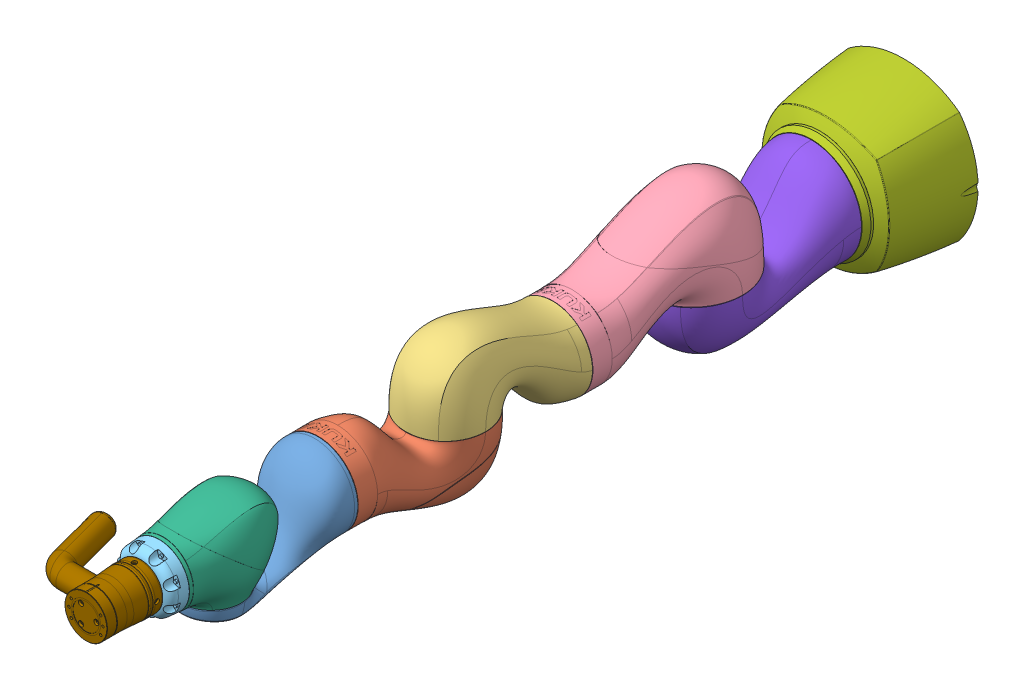
SolidWorks assembly lbrMed_withBaseLink_Frames, configuration Default. Lengths in mm.
Overall size (319.95 277.84 1446.36).
10 component instances, 10 part files, 6 mates.
Components (placement in the parent):
- Wrist1_body-2: Wrist1_body [Default] at origin size (137.43 170.81 261.47)
- UpperArm_body-1: UpperArm_body [Default] at origin size (137.03 183.96 286.04)
- Elbow_body-1: Elbow_body [Default] at origin size (136.09 183.95 261.22)
- LowerArm_body-1: LowerArm_body [Default] at origin size (171.08 201.65 323.93)
- Wrist3_body-1: Wrist3_body [Default] at origin size (102.25 102.25 38.4)
- Wrist2_body-1: Wrist2_body [Default] at origin size (136.25 137.94 182.79)
- Base_body-1: Base_body [Default] at origin size (277.84 277.84 157.78)
- Shoulder_body-1: Shoulder_body [Default] at origin size (171.08 202.96 299.34)
- only_platform-1: only_platform [Default] at (515.1468 0 -732.7058) x (-0.819152 0 -0.573576) z (0 1 0) size (1151.95 1181.08 766) (hidden)
- only_link-1: only_link [Default] at (515.1468 0 -732.7058) x (-0.819152 0 -0.573576) z (0 1 0) size (227.18 131.55 78.48)
Mates (geometry in assembly coordinates):
- Concentric1: concentric aligned: cylinder of Base_body-1 through (84.8528 84.8528 0) axis (0 0 1) radius 5; cylinder of only_platform-1 through (84.8528 84.8528 -125.779) axis (0 0 1) radius 5.25
- Concentric2: concentric aligned: cylinder of Base_body-1 through (84.8528 -84.8528 0) axis (0 0 1) radius 5; cylinder of only_platform-1 through (84.8528 -84.8528 -125.779) axis (0 0 1) radius 5.25
- Coincident1: coincident anti-aligned: plane of Base_body-1 through (0 0 3) normal (0 0 -1); plane of only_platform-1 through (127.5 127.5 3) normal (0 0 1)
- Concentric3: concentric anti-aligned: cylinder of Wrist3_body-1 through (-9.7581 9.7581 1289.3) axis (0 0 1) radius 3.2; cylinder of only_link-1 through (-9.7581 9.7581 1305.98) axis (0 0 -1) radius 3.2
- Concentric4: concentric anti-aligned: cylinder of Wrist3_body-1 through (9.7581 -9.7581 1289.3) axis (0 0 1) radius 3.2; cylinder of only_link-1 through (9.7581 -9.7581 1305.98) axis (0 0 -1) radius 3.2
- Coincident2: coincident anti-aligned: plane of Wrist3_body-1 through (0 30.5 1306) normal (0 0 1); plane of only_link-1 through (0 0 1306) normal (0 0 -1)
